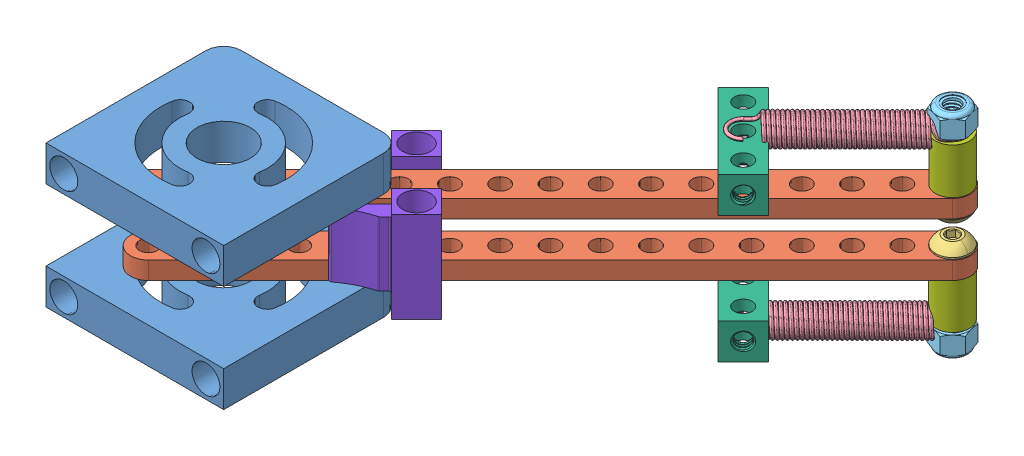
SolidWorks assembly Drone Launcher Assembly Spring Design, configuration Default. Lengths in mm.
Overall size (107.68 47.7 107.68).
17 component instances, 8 part files, 38 mates.
Components (placement in the parent):
- Drone Launcher Base-1: Drone Launcher Base [Default] at (9.5832 21.5969 33.0344) size (40 8 40)
- Drone Launcher Base-2: Drone Launcher Base [Default] at (9.5832 45.5969 33.0344) size (40 8 40)
- 17 hole flat beam.step-1: 17 hole flat beam.step [Default] at (46.3527 29.5969 -3.7352) x (0.707107 0 -0.707107) z (0.707107 0 0.707107) size (136 4 8)
- 17 hole flat beam.step-2: 17 hole flat beam.step [Default] at (46.3527 41.5969 -3.7352) x (0.707107 0 -0.707107) z (0.707107 0 0.707107) size (136 4 8)
- 14mm button head screw.step-1: 14mm button head screw.step [Default] at (91.6076 39.3969 -48.99) x (0.997884 0 -0.065013) z (0 -1 0) size (7.6 7.6 16.21)
- 14mm button head screw.step-2: 14mm button head screw.step [Default] at (91.6076 35.7969 -48.99) x (0.078916 0 -0.996881) z (0 1 0) size (7.6 7.6 16.21)
- 90404S.stp-1: 90404S.stp [Default] at (79.796 18.9607 -37.2375) x (0.708876 0 -0.705333) z (-0.705333 0 -0.708876) size (39.64 6.51 6.51)
  - EXTENSION.stp-1: EXTENSION.stp [Default] at origin size (39.64 6.51 6.51)
- 90404S.stp-3: 90404S.stp [Default] at (79.796 56.233 -37.2375) x (0.708876 0 -0.705333) z (0.705333 0 0.708876) size (39.64 6.51 6.51)
  - EXTENSION.stp-1: EXTENSION.stp [Default] at origin size (39.64 6.51 6.51)
- lock nut.step-1: lock nut.step [Default] at (91.6076 18.5946 -48.99) x (0.258819 0 -0.965926) z (-0.965926 0 -0.258819) size (7.02 4.86 8.1)
- 3 hole square beam.step-1: 3 hole square beam.step [Default] at (62.3275 23.3426 -31.1418) x (0.707107 0 -0.707107) z (0 -1 0) size (8 24.01 8)
- 3 hole square beam.step-3: 3 hole square beam.step [Default] at (62.3275 51.8511 -31.1418) x (-0.707107 0 0.707107) z (0 1 0) size (8 24.01 8)
- Spacer For Spring Launcher-1: Spacer For Spring Launcher [Default] at (91.6076 19.3269 -48.99) x (0.980554 0 0.196247) z (-0.196247 0 0.980554) size (7.6 10.27 7.6)
- Spacer For Spring Launcher-2: Spacer For Spring Launcher [Default] at (91.6076 45.5969 -48.99) x (0.959649 0 -0.281202) z (0.281202 0 0.959649) size (7.6 10.27 7.6)
- lock nut.step-2: lock nut.step [Default] at (91.6076 56.5991 -48.99) x (0.707107 0 0.707107) z (-0.707107 0 0.707107) size (7.02 4.86 8.1)
- New Bracket-2: New Bracket [Default] at (34.115 37.5969 8.5025) x (0 1 0) z (0.707107 0 0.707107) size (20.5 18 23.2)
Mates (geometry in assembly coordinates):
- Coincident1: coincident aligned: plane of Drone Launcher Base-1 through (-10.4168 29.5969 53.0344) normal (-1 0 0); plane of Drone Launcher Base-2 through (-10.4168 53.5969 53.0344) normal (-1 0 0)
- Coincident2: coincident aligned: plane of Drone Launcher Base-1 through (-10.4168 29.5969 53.0344) normal (0 0 1); plane of Drone Launcher Base-2 through (-10.4168 53.5969 53.0344) normal (0 0 1)
- Coincident5: coincident anti-aligned: plane of Drone Launcher Base-1 through (9.5832 29.5969 33.0344) normal (0 1 0); plane of 17 hole flat beam.step-1 through (1.0979 29.5969 41.5197) normal (0 -1 0)
- Parallel3: parallel aligned: plane of 17 hole flat beam.step-1 through (-1.7305 33.5969 38.6912) normal (-0.707107 0 -0.707107); plane of 17 hole flat beam.step-2 through (-1.7305 45.5969 38.6912) normal (-0.707107 0 -0.707107)
- Coincident7: coincident anti-aligned: plane of Drone Launcher Base-2 through (9.5832 45.5969 33.0344) normal (0 -1 0); plane of 17 hole flat beam.step-2 through (1.0979 45.5969 41.5197) normal (0 1 0)
- Coincident8: coincident aligned: plane of 17 hole flat beam.step-1 through (-1.7305 33.5969 38.6912) normal (-0.707107 0 -0.707107); plane of 17 hole flat beam.step-2 through (-1.7305 45.5969 38.6912) normal (-0.707107 0 -0.707107)
- Concentric8: concentric aligned: cylinder of 17 hole flat beam.step-1 through (1.0979 33.5969 41.5197) axis (0 1 0) radius 2; cylinder of 17 hole flat beam.step-2 through (1.0979 45.5969 41.5197) axis (0 1 0) radius 2
- Tangent5: tangent aligned: cylinder of Drone Launcher Base-2 through (9.5832 53.5969 33.0344) axis (0 -1 0) radius 6; cylinder of 17 hole flat beam.step-2 through (6.7547 45.5969 35.8628) axis (0 1 0) radius 2
- Tangent6: tangent aligned: cylinder of Drone Launcher Base-2 through (9.5832 53.5969 33.0344) axis (0 -1 0) radius 6; cylinder of 17 hole flat beam.step-2 through (12.4116 45.5969 30.206) axis (0 1 0) radius 2
- Distance2: distance = 24 mm: cylinder of Drone Launcher Base-1 through (-6.4168 25.5969 48.3344) axis (0 0 1) radius 3.15; cylinder of Drone Launcher Base-2 through (-6.4168 49.5969 48.3344) axis (0 0 1) radius 3.15
- Angle2: planar angle = 2.356194 rad anti-aligned: plane of 17 hole flat beam.step-2 through (-1.7305 45.5969 38.6912) normal (-0.707107 0 -0.707107); plane of Drone Launcher Base-2 through (-10.4168 53.5969 13.0344) normal (0 0 -1)
- Concentric12: concentric anti-aligned: cylinder of 17 hole flat beam.step-1 through (91.6076 33.5969 -48.99) axis (0 1 0) radius 2; circle of 14mm button head screw.step-1
- Coincident10: coincident anti-aligned: plane of 17 hole flat beam.step-2 through (1.0979 41.5969 41.5197) normal (0 -1 0); plane of 14mm button head screw.step-1 through (91.3605 41.5969 -52.782) normal (0 1 0)
- Concentric13: concentric aligned: cylinder of 17 hole flat beam.step-1 through (91.6076 33.5969 -48.99) axis (0 1 0) radius 2; circle of 14mm button head screw.step-2
- Coincident11: coincident anti-aligned: plane of 17 hole flat beam.step-1 through (1.0979 33.5969 41.5197) normal (0 1 0); plane of 14mm button head screw.step-2 through (95.3957 33.5969 -48.6901) normal (0 -1 0)
- Concentric23: concentric anti-aligned: circle of 90404S.stp-1/EXTENSION.stp-1; circle of 90404S.stp-3/EXTENSION.stp-1
- Tangent10: tangent anti-aligned: torus of 90404S.stp-1/EXTENSION.stp-1; plane of lock nut.step-1 through (95.5113 18.5946 -47.944) normal (0 1 0)
- Coincident26: coincident aligned: plane of 3 hole square beam.step-1 through (59.4991 23.3426 -33.9702) normal (-0.707107 0 -0.707107); plane of 3 hole square beam.step-3 through (59.4991 51.8511 -33.9702) normal (-0.707107 0 -0.707107)
- Parallel7: parallel aligned: plane of 17 hole flat beam.step-1 through (-1.7305 33.5969 38.6912) normal (-0.707107 0 -0.707107); plane of 3 hole square beam.step-1 through (59.4991 23.3426 -33.9702) normal (-0.707107 0 -0.707107)
- Coincident29: coincident aligned: plane of 3 hole square beam.step-1 through (62.3275 23.3426 -25.4849) normal (-0.707107 0 0.707107); plane of 3 hole square beam.step-3 through (62.3275 51.8511 -25.4849) normal (-0.707107 0 0.707107)
- Concentric26: concentric anti-aligned: circle of 90404S.stp-1/EXTENSION.stp-1; cylinder of 3 hole square beam.step-1 through (67.9844 27.3426 -25.4849) axis (0 1 0) radius 2
- Tangent11: tangent anti-aligned: torus of 90404S.stp-1/EXTENSION.stp-1; plane of 3 hole square beam.step-1 through (65.156 19.3426 -28.3134) normal (0 -1 0)
- Concentric27: concentric anti-aligned: circle of 17 hole flat beam.step-1; circle of 90404S.stp-1/EXTENSION.stp-1
- Concentric28: concentric anti-aligned: circle of 17 hole flat beam.step-1; cylinder of Spacer For Spring Launcher-1 through (91.6076 29.5969 -48.99) axis (0 -1 0) radius 3.8
- Tangent12: tangent anti-aligned: torus of 90404S.stp-1/EXTENSION.stp-1; plane of Spacer For Spring Launcher-1 through (91.6076 19.3269 -48.99) normal (0 -1 0)
- Concentric29: concentric anti-aligned: circle of 17 hole flat beam.step-2; cylinder of Spacer For Spring Launcher-2 through (91.6076 55.8669 -48.99) axis (0 -1 0) radius 3.8
- Concentric30: concentric anti-aligned: circle of 90404S.stp-3/EXTENSION.stp-1; cylinder of Spacer For Spring Launcher-2 through (91.6076 55.8669 -48.99) axis (0 -1 0) radius 3.8
- Tangent14: tangent anti-aligned: torus of 90404S.stp-3/EXTENSION.stp-1; plane of Spacer For Spring Launcher-2 through (91.6076 55.8669 -48.99) normal (0 1 0)
- Coincident37: coincident anti-aligned: plane of 17 hole flat beam.step-2 through (1.0979 45.5969 41.5197) normal (0 1 0); plane of Spacer For Spring Launcher-2 through (91.6076 45.5969 -48.99) normal (0 -1 0)
- Tangent15: tangent anti-aligned: torus of 90404S.stp-3/EXTENSION.stp-1; plane of lock nut.step-2 through (94.4653 56.5991 -51.8477) normal (0 -1 0)
- Concentric31: concentric aligned: circle of lock nut.step-1; cylinder of Spacer For Spring Launcher-1 through (91.6076 29.5969 -48.99) axis (0 -1 0) radius 3.8
- Concentric32: concentric aligned: cylinder of Spacer For Spring Launcher-2 through (91.6076 55.8669 -48.99) axis (0 -1 0) radius 3.8; circle of lock nut.step-2
- Coincident38: coincident aligned: plane of lock nut.step-1 through (87.7038 13.7446 -50.036) normal (-0.707107 0 -0.707107); plane of lock nut.step-2 through (90.5616 61.4491 -52.8937) normal (-0.707107 0 -0.707107)
- Parallel8: parallel aligned: plane of 17 hole flat beam.step-2 through (-1.7305 45.5969 38.6912) normal (-0.707107 0 -0.707107); plane of lock nut.step-2 through (90.5616 61.4491 -52.8937) normal (-0.707107 0 -0.707107)
- Tangent17: tangent anti-aligned: torus of 90404S.stp-3/EXTENSION.stp-1; plane of 3 hole square beam.step-3 through (65.156 55.8511 -28.3134) normal (0 1 0)
- Coincident42: coincident anti-aligned: plane of 17 hole flat beam.step-1 through (1.0979 29.5969 41.5197) normal (0 -1 0); circle of Spacer For Spring Launcher-1
- Distance7: distance = 0.4 mm anti-aligned: plane of 17 hole flat beam.step-2 through (1.0979 41.5969 41.5197) normal (0 -1 0); plane of New Bracket-2 through (31.5694 41.1969 17.2707) normal (0 1 0)
- Distance8: distance = 0.4 mm anti-aligned: plane of New Bracket-2 through (31.5694 47.8469 17.2707) normal (-0.707107 0 -0.707107); plane of 17 hole flat beam.step-2 through (3.9263 45.5969 44.3481) normal (0.707107 0 0.707107)
